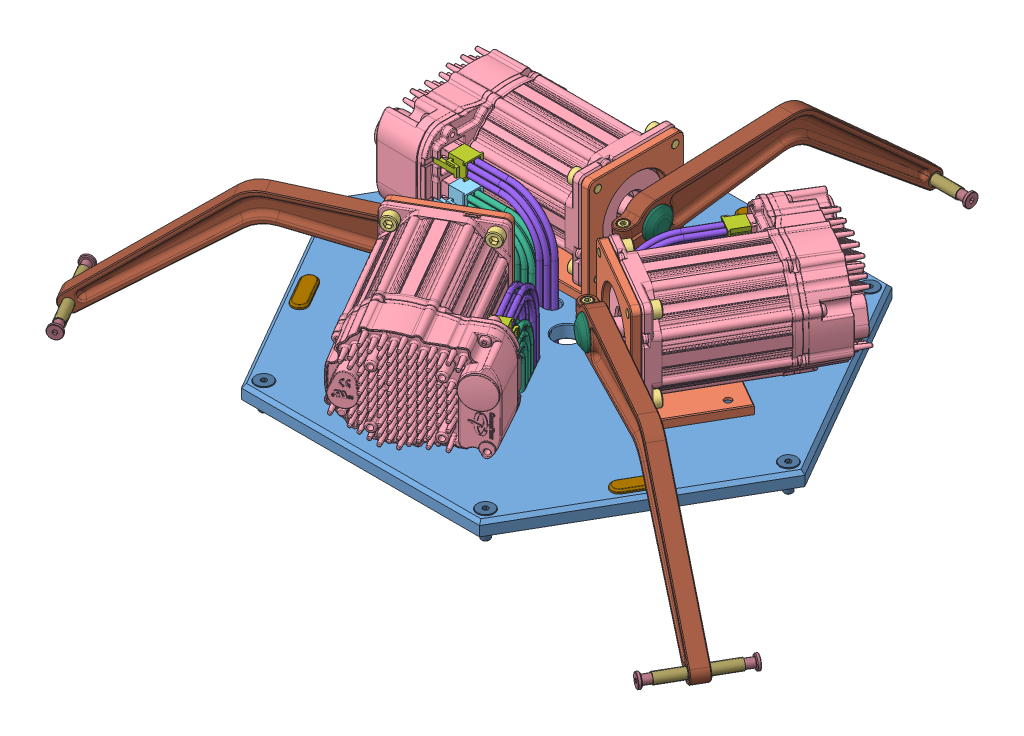
SolidWorks assembly top_plate_assembly, configuration Default. Lengths in mm.
Overall size (417.97 114.75 366.28).
85 component instances, 16 part files, 32 mates.
Components (placement in the parent):
- base_plate-1: base_plate [Default] at (-152.5992 184.5682 334.9696) size (290 8.05 251.15)
- motor_assembly-1: motor_assembly [Default] at (-130.6626 192.5682 338.9744) x (0.5 0 -0.866025) z (0 -1 0) size (124.71 82.13 99.26)
  - motor_angle_bracket-1: motor_angle_bracket [Default] at origin size (55 58 65)
  - socket head cap screw_am-1: socket head cap screw_am [B18.3.1M - 5 x 0.8 x 10 Hex SHCS -- 10NHX] at (14.819 52.5732 -59.5732) x (-1 0 0) z (0 -0.909932 -0.414757) size (15 8.5 8.5)
  - socket head cap screw_am-2: socket head cap screw_am [B18.3.1M - 5 x 0.8 x 10 Hex SHCS -- 10NHX] at (14.819 5.4268 -59.5732) x (-1 0 0) z (0 -0.909932 -0.414757) size (15 8.5 8.5)
  - socket head cap screw_am-3: socket head cap screw_am [B18.3.1M - 5 x 0.8 x 10 Hex SHCS -- 10NHX] at (14.819 5.4268 -12.4268) x (-1 0 0) z (0 -0.909932 -0.414757) size (15 8.5 8.5)
  - socket head cap screw_am-4: socket head cap screw_am [B18.3.1M - 5 x 0.8 x 10 Hex SHCS -- 10NHX] at (14.819 52.5732 -12.4268) x (-1 0 0) z (0 -0.909932 -0.414757) size (15 8.5 8.5)
  - CPM-_ _ _ _ -2321_-LS-1: CPM-_ _ _ _ -2321_-LS [Default] at (80.334 29 -36) x (0 1 0) z (1 0 0) size (82.13 59.99 124.71)
  - clearpath_data_loom-1: clearpath_data_loom [Default] at (61.0589 2.274 -42.6649) x (0 0 1) z (1 0 0) size (67.7 14.4 59.2)
    - 39-01-3085-1: 39-01-3085 [Default] at (15.1122 12.208 9.586) size (18 14.4 19.6)
    - microfit_4x2_loom-1: microfit_4x2_loom [Default] at (8.8122 10.183 -0.114) x (0 0 -1) z (1 0 0) size (40.6 7.9 66.6)
  - clearpath_power_loom-1: clearpath_power_loom [Default] at (70.645 -9.934 -48.6359) x (0 0 1) z (1 0 0) size (86.7 14.4 68.2)
    - 39-01-3045-1: 39-01-3045 [Default] at origin size (9.6 14.4 19.6)
    - microfit_2x2_loom-1: microfit_2x2_loom [Default] at (-2.1 -2.025 -9.7) x (0 0 -1) z (1 0 0) size (49.6 7.9 85.6)
- homing_block-1: homing_block [Default] at (-51.3492 192.5682 393.4263) x (0.5 0 -0.866025) z (0.866025 0 0.5) size (25 2 9)
- motor_assembly-2: motor_assembly [Default] at (-160.0992 192.5682 313.9696) x (-1 0 0) z (0 -1 0) size (124.71 82.13 99.26)
  - motor_angle_bracket-1: motor_angle_bracket [Default] at origin size (55 58 65)
  - socket head cap screw_am-1: socket head cap screw_am [B18.3.1M - 5 x 0.8 x 10 Hex SHCS -- 10NHX] at (14.819 52.5732 -59.5732) x (-1 0 0) z (0 -0.909932 -0.414757) size (15 8.5 8.5)
  - socket head cap screw_am-2: socket head cap screw_am [B18.3.1M - 5 x 0.8 x 10 Hex SHCS -- 10NHX] at (14.819 5.4268 -59.5732) x (-1 0 0) z (0 -0.909932 -0.414757) size (15 8.5 8.5)
  - socket head cap screw_am-3: socket head cap screw_am [B18.3.1M - 5 x 0.8 x 10 Hex SHCS -- 10NHX] at (14.819 5.4268 -12.4268) x (-1 0 0) z (0 -0.909932 -0.414757) size (15 8.5 8.5)
  - socket head cap screw_am-4: socket head cap screw_am [B18.3.1M - 5 x 0.8 x 10 Hex SHCS -- 10NHX] at (14.819 52.5732 -12.4268) x (-1 0 0) z (0 -0.909932 -0.414757) size (15 8.5 8.5)
  - CPM-_ _ _ _ -2321_-LS-1: CPM-_ _ _ _ -2321_-LS [Default] at (80.334 29 -36) x (0 1 0) z (1 0 0) size (82.13 59.99 124.71)
  - clearpath_data_loom-1: clearpath_data_loom [Default] at (61.0589 2.274 -42.6649) x (0 0 1) z (1 0 0) size (67.7 14.4 59.2)
    - 39-01-3085-1: 39-01-3085 [Default] at (15.1122 12.208 9.586) size (18 14.4 19.6)
    - microfit_4x2_loom-1: microfit_4x2_loom [Default] at (8.8122 10.183 -0.114) x (0 0 -1) z (1 0 0) size (40.6 7.9 66.6)
  - clearpath_power_loom-1: clearpath_power_loom [Default] at (70.645 -9.934 -48.6359) x (0 0 1) z (1 0 0) size (86.7 14.4 68.2)
    - 39-01-3045-1: 39-01-3045 [Default] at origin size (9.6 14.4 19.6)
    - microfit_2x2_loom-1: microfit_2x2_loom [Default] at (-2.1 -2.025 -9.7) x (0 0 -1) z (1 0 0) size (49.6 7.9 85.6)
- motor_assembly-3: motor_assembly [Default] at (-167.0357 192.5682 351.9648) x (0.5 0 0.866025) z (0 -1 0) size (124.71 82.13 99.26)
  - motor_angle_bracket-1: motor_angle_bracket [Default] at origin size (55 58 65)
  - socket head cap screw_am-1: socket head cap screw_am [B18.3.1M - 5 x 0.8 x 10 Hex SHCS -- 10NHX] at (14.819 52.5732 -59.5732) x (-1 0 0) z (0 -0.909932 -0.414757) size (15 8.5 8.5)
  - socket head cap screw_am-2: socket head cap screw_am [B18.3.1M - 5 x 0.8 x 10 Hex SHCS -- 10NHX] at (14.819 5.4268 -59.5732) x (-1 0 0) z (0 -0.909932 -0.414757) size (15 8.5 8.5)
  - socket head cap screw_am-3: socket head cap screw_am [B18.3.1M - 5 x 0.8 x 10 Hex SHCS -- 10NHX] at (14.819 5.4268 -12.4268) x (-1 0 0) z (0 -0.909932 -0.414757) size (15 8.5 8.5)
  - socket head cap screw_am-4: socket head cap screw_am [B18.3.1M - 5 x 0.8 x 10 Hex SHCS -- 10NHX] at (14.819 52.5732 -12.4268) x (-1 0 0) z (0 -0.909932 -0.414757) size (15 8.5 8.5)
  - CPM-_ _ _ _ -2321_-LS-1: CPM-_ _ _ _ -2321_-LS [Default] at (80.334 29 -36) x (0 1 0) z (1 0 0) size (82.13 59.99 124.71)
  - clearpath_data_loom-1: clearpath_data_loom [Default] at (61.0589 2.274 -42.6649) x (0 0 1) z (1 0 0) size (67.7 14.4 59.2)
    - 39-01-3085-1: 39-01-3085 [Default] at (15.1122 12.208 9.586) size (18 14.4 19.6)
    - microfit_4x2_loom-1: microfit_4x2_loom [Default] at (8.8122 10.183 -0.114) x (0 0 -1) z (1 0 0) size (40.6 7.9 66.6)
  - clearpath_power_loom-1: clearpath_power_loom [Default] at (70.645 -9.934 -48.6359) x (0 0 1) z (1 0 0) size (86.7 14.4 68.2)
    - 39-01-3045-1: 39-01-3045 [Default] at origin size (9.6 14.4 19.6)
    - microfit_2x2_loom-1: microfit_2x2_loom [Default] at (-2.1 -2.025 -9.7) x (0 0 -1) z (1 0 0) size (49.6 7.9 85.6)
- homing_block-2: homing_block [Default] at (-152.5992 192.5682 218.0562) x (-1 0 0) z (0 0 -1) size (25 2 9)
- homing_block-3: homing_block [Default] at (-253.8492 192.5682 393.4263) x (0.5 0 0.866025) z (-0.866025 0 0.5) size (25 2 9)
- socket countersunk head screw_am-1: socket countersunk head screw_am [B18.3.5M - 5 x 0.8 x 12 Socket FCHS  -- 12N] at (-205.0992 184.1682 307.4696) x (0 1 0) z (0 0 1) size (12 9.75 9.75)
- socket countersunk head screw_am-2: socket countersunk head screw_am [B18.3.5M - 5 x 0.8 x 12 Socket FCHS  -- 12N] at (-170.0992 184.1682 307.4696) x (0 1 0) z (0 0 1) size (12 9.75 9.75)
- socket countersunk head screw_am-3: socket countersunk head screw_am [B18.3.5M - 5 x 0.8 x 12 Socket FCHS  -- 12N] at (-170.0992 184.1682 262.4696) x (0 1 0) z (0 0 1) size (12 9.75 9.75)
- socket countersunk head screw_am-4: socket countersunk head screw_am [B18.3.5M - 5 x 0.8 x 12 Socket FCHS  -- 12N] at (-205.0992 184.1682 262.4696) x (0 1 0) z (0 0 1) size (12 9.75 9.75)
- socket countersunk head screw_am-5: socket countersunk head screw_am [B18.3.5M - 5 x 0.8 x 12 Socket FCHS  -- 12N] at (-120.0335 184.1682 333.5641) x (0 1 0) z (0 0 1) size (12 9.75 9.75)
- socket countersunk head screw_am-6: socket countersunk head screw_am [B18.3.5M - 5 x 0.8 x 12 Socket FCHS  -- 12N] at (-81.0623 184.1682 356.0641) x (0 1 0) z (0 0 1) size (12 9.75 9.75)
- socket countersunk head screw_am-7: socket countersunk head screw_am [B18.3.5M - 5 x 0.8 x 12 Socket FCHS  -- 12N] at (-63.5623 184.1682 325.7532) x (0 1 0) z (0 0 1) size (12 9.75 9.75)
- socket countersunk head screw_am-8: socket countersunk head screw_am [B18.3.5M - 5 x 0.8 x 12 Socket FCHS  -- 12N] at (-102.5335 184.1682 303.2532) x (0 1 0) z (0 0 1) size (12 9.75 9.75)
- socket countersunk head screw_am-9: socket countersunk head screw_am [B18.3.5M - 5 x 0.8 x 12 Socket FCHS  -- 12N] at (-167.6649 184.1682 363.875) x (0 1 0) z (0 0 1) size (12 9.75 9.75)
- socket countersunk head screw_am-10: socket countersunk head screw_am [B18.3.5M - 5 x 0.8 x 12 Socket FCHS  -- 12N] at (-150.1649 184.1682 394.1859) x (0 1 0) z (0 0 1) size (12 9.75 9.75)
- socket countersunk head screw_am-11: socket countersunk head screw_am [B18.3.5M - 5 x 0.8 x 12 Socket FCHS  -- 12N] at (-189.136 184.1682 416.6859) x (0 1 0) z (0 0 1) size (12 9.75 9.75)
- socket countersunk head screw_am-12: socket countersunk head screw_am [B18.3.5M - 5 x 0.8 x 12 Socket FCHS  -- 12N] at (-206.636 184.1682 386.375) x (0 1 0) z (0 0 1) size (12 9.75 9.75)
- socket countersunk head screw_am-13: socket countersunk head screw_am [B18.3.5M - 5 x 0.8 x 16 Socket FCHS  -- 16N] at (-287.5992 192.9682 334.9696) x (0 -1 0) z (0 0 1) size (16 9.75 9.75)
- socket countersunk head screw_am-14: socket countersunk head screw_am [B18.3.5M - 5 x 0.8 x 16 Socket FCHS  -- 16N] at (-220.0992 192.9682 451.883) x (0 -1 0) z (0 0 1) size (16 9.75 9.75)
- socket countersunk head screw_am-15: socket countersunk head screw_am [B18.3.5M - 5 x 0.8 x 16 Socket FCHS  -- 16N] at (-85.0992 192.9682 451.883) x (0 -1 0) z (0 0 1) size (16 9.75 9.75)
- socket countersunk head screw_am-16: socket countersunk head screw_am [B18.3.5M - 5 x 0.8 x 16 Socket FCHS  -- 16N] at (-17.5992 192.9682 334.9696) x (0 -1 0) z (0 0 1) size (16 9.75 9.75)
- socket countersunk head screw_am-17: socket countersunk head screw_am [B18.3.5M - 5 x 0.8 x 16 Socket FCHS  -- 16N] at (-85.0992 192.9682 218.0562) x (0 -1 0) z (0 0 1) size (16 9.75 9.75)
- socket countersunk head screw_am-18: socket countersunk head screw_am [B18.3.5M - 5 x 0.8 x 16 Socket FCHS  -- 16N] at (-220.0992 192.9682 218.0562) x (0 -1 0) z (0 0 1) size (16 9.75 9.75)
- bicep_assembly-1: bicep_assembly [Default] at (-157.5992 228.5682 284.9696) x (0 0.087592 -0.996156) z (0 -0.996156 -0.087592) size (188.86 55 93.71)
  - bicep2-1: bicep2 [Default] at origin size (188.72 10.11 93.57)
  - socket head cap screw_am-1: socket head cap screw_am [B18.3.1M - 3 x 0.5 x 10 Hex SHCS -- 10NHX] at (-15.0871 5 -6.5) x (0 0 1) z (-1 0 0) size (13 5.5 5.5)
  - bicep_elbow-1: bicep_elbow [Default] at (163.1354 5 76.0713) x (0.108786 0 0.994065) z (-0.994065 0 0.108786) size (7.5 41 7.5)
  - BGSP5-8-L5-1: BGSP5-8-L5 [Default] at (163.1354 -20.5 76.0713) x (0 1 0) z (0.821358 0 -0.570413) size (13 8 8)
  - BGSP5-8-L5-2: BGSP5-8-L5 [Default] at (163.1354 30.5 76.0713) x (0 -1 0) z (-0.767141 0 0.641478) size (13 8 8)
  - KES3_12-1: KES3_12 [Default] at (3.27 10.2126 1.5) x (0 -1 0) z (1 0 0) size (12 3 3)
  - servo_shaft_cover-1: servo_shaft_cover [Default] at (0 10 0) x (0 0 -1) z (1 0 0) size (18 4 18)
- bicep_assembly-2: bicep_assembly [Default] at (-106.7979 228.5682 355.6395) x (0.864095 0.066737 0.498885) z (0.057796 -0.997771 0.033368) size (188.86 55 93.71)
  - bicep2-1: bicep2 [Default] at origin size (188.72 10.11 93.57)
  - socket head cap screw_am-1: socket head cap screw_am [B18.3.1M - 3 x 0.5 x 10 Hex SHCS -- 10NHX] at (-15.0871 5 -6.5) x (0 0 1) z (-1 0 0) size (13 5.5 5.5)
  - bicep_elbow-1: bicep_elbow [Default] at (163.1354 5 76.0713) x (0.108786 0 0.994065) z (-0.994065 0 0.108786) size (7.5 41 7.5)
  - BGSP5-8-L5-1: BGSP5-8-L5 [Default] at (163.1354 -20.5 76.0713) x (0 1 0) z (0.821358 0 -0.570413) size (13 8 8)
  - BGSP5-8-L5-2: BGSP5-8-L5 [Default] at (163.1354 30.5 76.0713) x (0 -1 0) z (-0.767141 0 0.641478) size (13 8 8)
  - KES3_12-1: KES3_12 [Default] at (3.27 10.2126 1.5) x (0 -1 0) z (1 0 0) size (12 3 3)
  - servo_shaft_cover-1: servo_shaft_cover [Default] at (0 10 0) x (0 0 -1) z (1 0 0) size (18 4 18)
- bicep_assembly-3: bicep_assembly [Default] at (-193.4004 228.5682 364.2997) x (-0.860309 0.114705 0.4967) z (-0.099338 -0.9934 0.057353) size (188.86 55 93.71)
  - bicep2-1: bicep2 [Default] at origin size (188.72 10.11 93.57)
  - socket head cap screw_am-1: socket head cap screw_am [B18.3.1M - 3 x 0.5 x 10 Hex SHCS -- 10NHX] at (-15.0871 5 -6.5) x (0 0 1) z (-1 0 0) size (13 5.5 5.5)
  - bicep_elbow-1: bicep_elbow [Default] at (163.1354 5 76.0713) x (0.108786 0 0.994065) z (-0.994065 0 0.108786) size (7.5 41 7.5)
  - BGSP5-8-L5-1: BGSP5-8-L5 [Default] at (163.1354 -20.5 76.0713) x (0 1 0) z (0.821358 0 -0.570413) size (13 8 8)
  - BGSP5-8-L5-2: BGSP5-8-L5 [Default] at (163.1354 30.5 76.0713) x (0 -1 0) z (-0.767141 0 0.641478) size (13 8 8)
  - KES3_12-1: KES3_12 [Default] at (3.27 10.2126 1.5) x (0 -1 0) z (1 0 0) size (12 3 3)
  - servo_shaft_cover-1: servo_shaft_cover [Default] at (0 10 0) x (0 0 -1) z (1 0 0) size (18 4 18)
Mates (geometry in assembly coordinates):
- Coincident2: coincident anti-aligned: plane of base_plate-1 through (-152.5992 192.5682 334.9696) normal (0 1 0); plane of motor_assembly-1/motor_angle_bracket-1 through (-52.9332 192.5682 320.343) normal (0 -1 0)
- Concentric2: concentric aligned: cylinder of base_plate-1 through (-81.0623 184.5682 356.0641) axis (0 -1 0) radius 2.75; cylinder of motor_assembly-1/motor_angle_bracket-1 through (-81.0623 192.5682 356.0641) axis (0 -1 0) radius 2.1
- Concentric3: concentric aligned: cylinder of base_plate-1 through (-120.0335 184.5682 333.5641) axis (0 -1 0) radius 2.75; cylinder of motor_assembly-1/motor_angle_bracket-1 through (-120.0335 192.5682 333.5641) axis (0 -1 0) radius 2.1
- Coincident3: coincident anti-aligned: plane of base_plate-1 through (-152.5992 192.5682 334.9696) normal (0 1 0); plane of homing_block-1 through (-55.3492 192.5682 400.3545) normal (0 -1 0)
- Concentric4: concentric aligned: cylinder of base_plate-1 through (-55.3492 192.5682 400.3545) axis (0 1 0) radius 1.25; cylinder of homing_block-1 through (-55.3492 192.5682 400.3545) axis (0 1 0) radius 1.25
- Concentric5: concentric aligned: cylinder of base_plate-1 through (-47.3492 192.5682 386.4981) axis (0 1 0) radius 1.25; cylinder of homing_block-1 through (-47.3492 192.5682 386.4981) axis (0 1 0) radius 1.25
- Coincident18: coincident aligned: cone of base_plate-1 through (-205.0992 184.5682 307.4696) axis (0 1 0); cone of socket countersunk head screw_am-1 through (-205.0992 184.8932 307.4696) axis (0 1 0)
- Coincident19: coincident aligned: cone of base_plate-1 through (-170.0992 184.5682 307.4696) axis (0 1 0); cone of socket countersunk head screw_am-2 through (-170.0992 184.8932 307.4696) axis (0 1 0)
- Coincident20: coincident aligned: cone of base_plate-1 through (-170.0992 184.5682 262.4696) axis (0 1 0); cone of socket countersunk head screw_am-3 through (-170.0992 184.8932 262.4696) axis (0 1 0)
- Coincident21: coincident aligned: cone of base_plate-1 through (-205.0992 184.5682 262.4696) axis (0 1 0); cone of socket countersunk head screw_am-4 through (-205.0992 184.8932 262.4696) axis (0 1 0)
- Coincident22: coincident aligned: cone of base_plate-1 through (-120.0335 184.5682 333.5641) axis (0 1 0); cone of socket countersunk head screw_am-5 through (-120.0335 184.8932 333.5641) axis (0 1 0)
- Coincident23: coincident aligned: cone of base_plate-1 through (-81.0623 184.5682 356.0641) axis (0 1 0); cone of socket countersunk head screw_am-6 through (-81.0623 184.8932 356.0641) axis (0 1 0)
- Coincident24: coincident aligned: cone of base_plate-1 through (-63.5623 184.5682 325.7532) axis (0 1 0); cone of socket countersunk head screw_am-7 through (-63.5623 184.8932 325.7532) axis (0 1 0)
- Coincident25: coincident aligned: cone of base_plate-1 through (-102.5335 184.5682 303.2532) axis (0 1 0); cone of socket countersunk head screw_am-8 through (-102.5335 184.8932 303.2532) axis (0 1 0)
- Coincident26: coincident aligned: cone of base_plate-1 through (-167.6649 184.5682 363.875) axis (0 1 0); cone of socket countersunk head screw_am-9 through (-167.6649 184.8932 363.875) axis (0 1 0)
- Coincident27: coincident aligned: cone of base_plate-1 through (-150.1649 184.5682 394.1859) axis (0 1 0); cone of socket countersunk head screw_am-10 through (-150.1649 184.8932 394.1859) axis (0 1 0)
- Coincident28: coincident aligned: cone of base_plate-1 through (-189.136 184.5682 416.6859) axis (0 1 0); cone of socket countersunk head screw_am-11 through (-189.136 184.8932 416.6859) axis (0 1 0)
- Coincident29: coincident aligned: cone of base_plate-1 through (-206.636 184.5682 386.375) axis (0 1 0); cone of socket countersunk head screw_am-12 through (-206.636 184.8932 386.375) axis (0 1 0)
- Concentric301: concentric aligned: cylinder of homing_block-1 through (-55.3492 192.5682 400.3545) axis (0 1 0) radius 1.25; cylinder of ? through (-55.3492 196.2182 400.3545) axis (0 1 0) radius 1.5
- Coincident521: coincident anti-aligned: plane of homing_block-1 through (-55.3492 194.5682 400.3545) normal (0 1 0); plane of ? through (-53.8492 194.5682 400.3545) normal (0 -1 0)
- Coincident62: coincident aligned: cone of base_plate-1 through (-287.5992 192.5682 334.9696) axis (0 -1 0); cone of socket countersunk head screw_am-13 through (-287.5992 192.2432 334.9696) axis (0 -1 0)
- Coincident63: coincident aligned: cone of base_plate-1 through (-220.0992 192.5682 451.883) axis (0 -1 0); cone of socket countersunk head screw_am-14 through (-220.0992 192.2432 451.883) axis (0 -1 0)
- Coincident64: coincident aligned: cone of base_plate-1 through (-85.0992 192.5682 451.883) axis (0 -1 0); cone of socket countersunk head screw_am-15 through (-85.0992 192.2432 451.883) axis (0 -1 0)
- Coincident65: coincident aligned: cone of base_plate-1 through (-17.5992 192.5682 334.9696) axis (0 -1 0); cone of socket countersunk head screw_am-16 through (-17.5992 192.2432 334.9696) axis (0 -1 0)
- Coincident66: coincident aligned: cone of base_plate-1 through (-85.0992 192.5682 218.0562) axis (0 -1 0); cone of socket countersunk head screw_am-17 through (-85.0992 192.2432 218.0562) axis (0 -1 0)
- Coincident67: coincident aligned: cone of base_plate-1 through (-220.0992 192.5682 218.0562) axis (0 -1 0); cone of socket countersunk head screw_am-18 through (-220.0992 192.2432 218.0562) axis (0 -1 0)
- Concentric332: concentric anti-aligned: cylinder of motor_assembly-2/CPM-_ _ _ _ -2321_-LS-1 through (-113.9579 228.5682 284.9696) axis (1 0 0) radius 4.7625; cylinder of bicep_assembly-1/bicep2-1 through (-147.5992 228.5682 284.9696) axis (-1 0 0) radius 4.77
- Concentric333: concentric anti-aligned: cylinder of motor_assembly-1/CPM-_ _ _ _ -2321_-LS-1 through (-128.6186 228.5682 393.4339) axis (-0.5 0 0.866025) radius 4.7625; cylinder of bicep_assembly-2/bicep2-1 through (-111.7979 228.5682 364.2997) axis (0.5 0 -0.866025) radius 4.77
- Concentric334: concentric anti-aligned: cylinder of motor_assembly-3/CPM-_ _ _ _ -2321_-LS-1 through (-215.2211 228.5682 326.5052) axis (-0.5 0 -0.866025) radius 4.7625; cylinder of bicep_assembly-3/bicep2-1 through (-198.4004 228.5682 355.6395) axis (0.5 0 0.866025) radius 4.77
- Width1: width: plane of bicep_assembly-1/bicep2-1 through (-147.5992 228.5682 284.9696) normal (1 0 0); plane of bicep_assembly-1/bicep2-1 through (-157.5992 228.5682 284.9696) normal (-1 0 0); cylinder of base_plate-1 through (-152.5992 184.5682 334.9696) axis (0 1 0) radius 7.5
- Width2: width: plane of bicep_assembly-2/bicep2-1 through (-111.7979 228.5682 364.2997) normal (-0.5 0 0.866025); plane of bicep_assembly-2/bicep2-1 through (-106.7979 228.5682 355.6395) normal (0.5 0 -0.866025); cylinder of base_plate-1 through (-152.5992 184.5682 334.9696) axis (0 1 0) radius 7.5
- Width3: width: plane of bicep_assembly-3/bicep2-1 through (-193.4004 228.5682 364.2997) normal (0.5 0 0.866025); plane of bicep_assembly-3/bicep2-1 through (-198.4004 228.5682 355.6395) normal (-0.5 0 -0.866025); cylinder of base_plate-1 through (-152.5992 184.5682 334.9696) axis (0 1 0) radius 7.5
